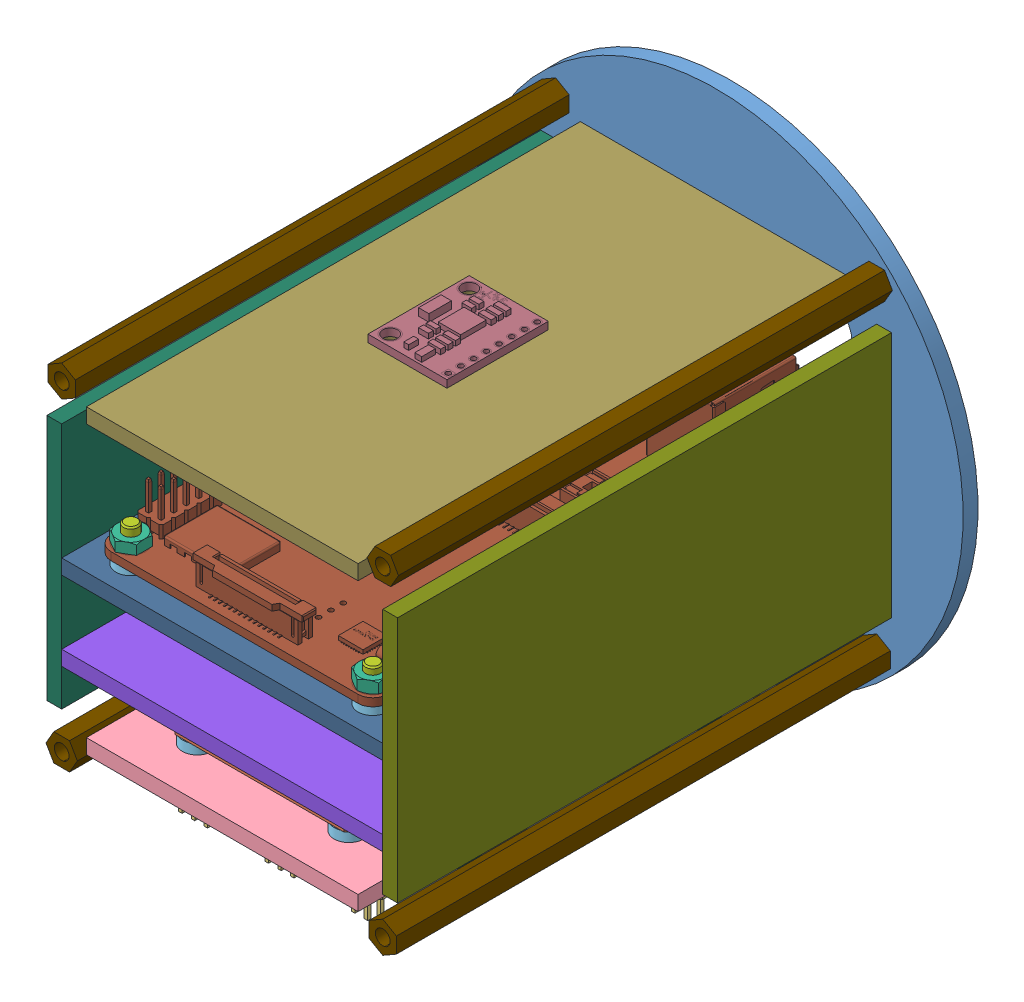
SolidWorks assembly Сборка4, configuration По умолчанию. Lengths in mm.
Overall size (100 100 104.65).
127 component instances, 20 part files, 170 mates.
Components (placement in the parent):
- baze-100mm-1: baze-100mm [По умолчанию] at origin size (100 100 3)
- Matek Power Hub-2: Matek Power Hub [По умолчанию] at (0.0123 -25.5 28.6623) x (0 0 -1) z (1 0 0) size (36.25 3.92 36.25)
- ACS712.step-1: ACS712.step [По умолчанию] at (17.5 -32.5 27.745) x (0 0 1) z (1 0 0) size (31.19 12.78 13.3)
- ACS712.step-2: ACS712.step [По умолчанию] at (0 -32.5 27.745) x (0 0 1) z (1 0 0) size (31.19 12.78 13.3)
- ACS712.step-3: ACS712.step [По умолчанию] at (-17.5 -32.5 27.745) x (0 0 1) z (1 0 0) size (31.19 12.78 13.3)
- level-0-1: level-0 [По умолчанию] at (0 -30.5 53) x (1 0 0) z (0 1 0) size (55 103 3)
- Matek Power Hub-4: Matek Power Hub [По умолчанию] at (0.0123 -25.5 77.3623) size (36.25 3.92 36.25)
- ACS712.step-7: ACS712.step [По умолчанию] at (17.5 -32.5 78.255) x (0 0 -1) z (-1 0 0) size (31.19 12.78 13.3)
- ACS712.step-8: ACS712.step [По умолчанию] at (0 -32.5 78.255) x (0 0 -1) z (-1 0 0) size (31.19 12.78 13.3)
- ACS712.step-9: ACS712.step [По умолчанию] at (-17.5 -32.5 78.255) x (0 0 -1) z (-1 0 0) size (31.19 12.78 13.3)
- 3-6-3-1: 3-6-3 [По умолчанию] at (15.35 -27.5 92.7) x (0.999975 0 -0.007062) z (0 1 0) size (6 6 2)
- 3-6-3-2: 3-6-3 [По умолчанию] at (-15.35 -27.5 92.7) x (0.992437 0 -0.122755) z (0 1 0) size (6 6 2)
- 3-6-3-3: 3-6-3 [По умолчанию] at (15.35 -27.5 62) x (0.931904 0 -0.362706) z (0 1 0) size (6 6 2)
- 3-6-3-4: 3-6-3 [По умолчанию] at (-15.35 -27.5 62) x (1 0 0) z (0 1 0) size (6 6 2)
- hex nut style 1 gradeab_iso-1: hex nut style 1 gradeab_iso [ISO - 4032 - M3 - D - N] at (15.3745 -21.9 62) x (1 0 0) z (0 1 0) size (5.5 6.35 2.4)
- hex nut style 1 gradeab_iso-2: hex nut style 1 gradeab_iso [ISO - 4032 - M3 - D - N] at (-15.35 -21.9 62) x (1 0 0) z (0 1 0) size (5.5 6.35 2.4)
- hex nut style 1 gradeab_iso-3: hex nut style 1 gradeab_iso [ISO - 4032 - M3 - D - N] at (15.3745 -21.9 92.7245) x (1 0 0) z (0 1 0) size (5.5 6.35 2.4)
- hex nut style 1 gradeab_iso-4: hex nut style 1 gradeab_iso [ISO - 4032 - M3 - D - N] at (-15.35 -21.9 92.7245) x (1 0 0) z (0 1 0) size (5.5 6.35 2.4)
- hex nut style 1 gradeab_iso-5: hex nut style 1 gradeab_iso [ISO - 4032 - M3 - D - N] at (15.3745 -21.9 44.0245) x (1 0 0) z (0 1 0) size (5.5 6.35 2.4)
- hex nut style 1 gradeab_iso-6: hex nut style 1 gradeab_iso [ISO - 4032 - M3 - D - N] at (-15.35 -21.9 44.0245) x (1 0 0) z (0 1 0) size (5.5 6.35 2.4)
- hex nut style 1 gradeab_iso-7: hex nut style 1 gradeab_iso [ISO - 4032 - M3 - D - N] at (15.3745 -21.9 13.3) x (1 0 0) z (0 1 0) size (5.5 6.35 2.4)
- hex nut style 1 gradeab_iso-8: hex nut style 1 gradeab_iso [ISO - 4032 - M3 - D - N] at (-15.35 -21.9 13.3) x (1 0 0) z (0 1 0) size (5.5 6.35 2.4)
- socket countersunk head screw_iso-1: socket countersunk head screw_iso [ISO 10642 - M3 x 8 - 8N] at (15.35 -30.11 92.7) x (0 1 0) z (-0.074206 0 0.997243) size (8 5.54 5.54)
- socket countersunk head screw_iso-2: socket countersunk head screw_iso [ISO 10642 - M3 x 8 - 8N] at (15.35 -30.11 62) x (0 1 0) z (-0.12314 0 0.992389) size (8 5.54 5.54)
- socket countersunk head screw_iso-3: socket countersunk head screw_iso [ISO 10642 - M3 x 8 - 8N] at (-15.35 -30.11 62) x (0 1 0) z (-0.109262 0 0.994013) size (8 5.54 5.54)
- socket countersunk head screw_iso-4: socket countersunk head screw_iso [ISO 10642 - M3 x 8 - 8N] at (-15.35 -30.11 92.7) x (0 1 0) z (-0.069269 0 0.997598) size (8 5.54 5.54)
- socket countersunk head screw_iso-5: socket countersunk head screw_iso [ISO 10642 - M3 x 8 - 8N] at (-22.5 -27.89 77.35) x (0 -1 0) z (-0.066693 0 0.997774) size (8 5.54 5.54)
- socket countersunk head screw_iso-6: socket countersunk head screw_iso [ISO 10642 - M3 x 8 - 8N] at (-12.5 -27.89 77.35) x (0 -1 0) z (-0.00561 0 0.999984) size (8 5.54 5.54)
- socket countersunk head screw_iso-7: socket countersunk head screw_iso [ISO 10642 - M3 x 8 - 8N] at (-5 -27.89 77.35) x (0 -1 0) z (0.004518 0 0.99999) size (8 5.54 5.54)
- socket countersunk head screw_iso-8: socket countersunk head screw_iso [ISO 10642 - M3 x 8 - 8N] at (5 -27.89 77.35) x (0 -1 0) z (0.047845 0 0.998855) size (8 5.54 5.54)
- socket countersunk head screw_iso-9: socket countersunk head screw_iso [ISO 10642 - M3 x 8 - 8N] at (12.5 -27.89 77.35) x (0 -1 0) z (0.031705 0 0.999497) size (8 5.54 5.54)
- socket countersunk head screw_iso-10: socket countersunk head screw_iso [ISO 10642 - M3 x 8 - 8N] at (22.5 -27.89 77.35) x (0 -1 0) z (0.037692 0 0.999289) size (8 5.54 5.54)
- hex nut style 1 gradeab_iso-13: hex nut style 1 gradeab_iso [ISO - 4032 - M3 - D - N] at (22.5 -36.48 77.35) x (1 0 0) z (0 -1 0) size (5.5 6.35 2.4)
- hex nut style 1 gradeab_iso-14: hex nut style 1 gradeab_iso [ISO - 4032 - M3 - D - N] at (12.5 -36.48 77.35) x (1 0 0) z (0 -1 0) size (5.5 6.35 2.4)
- hex nut style 1 gradeab_iso-15: hex nut style 1 gradeab_iso [ISO - 4032 - M3 - D - N] at (5 -36.48 77.35) x (1 0 0) z (0 -1 0) size (5.5 6.35 2.4)
- hex nut style 1 gradeab_iso-16: hex nut style 1 gradeab_iso [ISO - 4032 - M3 - D - N] at (-5 -36.48 77.35) x (1 0 0) z (0 -1 0) size (5.5 6.35 2.4)
- hex nut style 1 gradeab_iso-17: hex nut style 1 gradeab_iso [ISO - 4032 - M3 - D - N] at (-12.5 -36.48 77.35) x (1 0 0) z (0 -1 0) size (5.5 6.35 2.4)
- hex nut style 1 gradeab_iso-18: hex nut style 1 gradeab_iso [ISO - 4032 - M3 - D - N] at (-22.5 -36.48 77.35) x (1 0 0) z (0 -1 0) size (5.5 6.35 2.4)
- 3-6-3-5: 3-6-3 [По умолчанию] at (22.5 -32.5 77.35) x (1 0 0) z (0 1 0) size (6 6 2)
- 3-6-3-6: 3-6-3 [По умолчанию] at (12.5 -32.5 77.35) x (1 0 0) z (0 1 0) size (6 6 2)
- 3-6-3-7: 3-6-3 [По умолчанию] at (5 -32.5 77.35) x (1 0 0) z (0 1 0) size (6 6 2)
- 3-6-3-8: 3-6-3 [По умолчанию] at (-5 -32.5 77.35) x (1 0 0) z (0 1 0) size (6 6 2)
- 3-6-3-9: 3-6-3 [По умолчанию] at (-12.5 -32.5 77.35) x (1 0 0) z (0 1 0) size (6 6 2)
- 3-6-3-10: 3-6-3 [По умолчанию] at (-22.5 -32.5 77.35) x (1 0 0) z (0 1 0) size (6 6 2)
- 3-6-3-11: 3-6-3 [По умолчанию] at (-22.5 -30.5 28.65) x (1 0 0) z (0 -1 0) size (6 6 2)
- hex nut style 1 gradeab_iso-19: hex nut style 1 gradeab_iso [ISO - 4032 - M3 - D - N] at (-22.5 -34.08 28.65) x (1 0 0) z (0 1 0) size (5.5 6.35 2.4)
- hex nut style 1 gradeab_iso-20: hex nut style 1 gradeab_iso [ISO - 4032 - M3 - D - N] at (-12.5 -34.08 28.65) x (1 0 0) z (0 1 0) size (5.5 6.35 2.4)
- 3-6-3-12: 3-6-3 [По умолчанию] at (-12.5 -30.5 28.65) x (1 0 0) z (0 -1 0) size (6 6 2)
- hex nut style 1 gradeab_iso-21: hex nut style 1 gradeab_iso [ISO - 4032 - M3 - D - N] at (-5 -34.08 28.65) x (1 0 0) z (0 1 0) size (5.5 6.35 2.4)
- hex nut style 1 gradeab_iso-22: hex nut style 1 gradeab_iso [ISO - 4032 - M3 - D - N] at (5 -34.08 28.65) x (1 0 0) z (0 1 0) size (5.5 6.35 2.4)
- hex nut style 1 gradeab_iso-23: hex nut style 1 gradeab_iso [ISO - 4032 - M3 - D - N] at (12.5 -34.08 28.65) x (1 0 0) z (0 1 0) size (5.5 6.35 2.4)
- hex nut style 1 gradeab_iso-24: hex nut style 1 gradeab_iso [ISO - 4032 - M3 - D - N] at (22.5 -34.08 28.65) x (1 0 0) z (0 1 0) size (5.5 6.35 2.4)
- socket countersunk head screw_iso-11: socket countersunk head screw_iso [ISO 10642 - M3 x 8 - 8N] at (22.5 -27.89 28.65) x (0 -1 0) z (-0.037692 0 0.999289) size (8 5.54 5.54)
- socket countersunk head screw_iso-12: socket countersunk head screw_iso [ISO 10642 - M3 x 8 - 8N] at (12.5 -27.89 28.65) x (0 -1 0) z (-0.031705 0 0.999497) size (8 5.54 5.54)
- socket countersunk head screw_iso-13: socket countersunk head screw_iso [ISO 10642 - M3 x 8 - 8N] at (5 -27.89 28.65) x (0 -1 0) z (-0.047845 0 0.998855) size (8 5.54 5.54)
- socket countersunk head screw_iso-14: socket countersunk head screw_iso [ISO 10642 - M3 x 8 - 8N] at (-5 -27.89 28.65) x (0 -1 0) z (-0.004518 0 0.99999) size (8 5.54 5.54)
- socket countersunk head screw_iso-15: socket countersunk head screw_iso [ISO 10642 - M3 x 8 - 8N] at (-12.5 -27.89 28.65) x (0 -1 0) z (0.00561 0 0.999984) size (8 5.54 5.54)
- socket countersunk head screw_iso-16: socket countersunk head screw_iso [ISO 10642 - M3 x 8 - 8N] at (-22.5 -27.89 28.65) x (0 -1 0) z (0.066693 0 0.997774) size (8 5.54 5.54)
- 3-6-3-13: 3-6-3 [По умолчанию] at (-5 -30.5 28.65) x (1 0 0) z (0 -1 0) size (6 6 2)
- 3-6-3-14: 3-6-3 [По умолчанию] at (5 -30.5 28.65) x (1 0 0) z (0 -1 0) size (6 6 2)
- 3-6-3-15: 3-6-3 [По умолчанию] at (12.5 -30.5 28.65) x (1 0 0) z (0 -1 0) size (6 6 2)
- 3-6-3-16: 3-6-3 [По умолчанию] at (22.5 -30.5 28.65) x (1 0 0) z (0 -1 0) size (6 6 2)
- socket countersunk head screw_iso-17: socket countersunk head screw_iso [ISO 10642 - M3 x 8 - 8N] at (-15.35 -30.11 13.3) x (0 1 0) z (0.069269 0 0.997598) size (8 5.54 5.54)
- socket countersunk head screw_iso-18: socket countersunk head screw_iso [ISO 10642 - M3 x 8 - 8N] at (15.35 -30.11 13.3) x (0 1 0) z (0.074206 0 0.997243) size (8 5.54 5.54)
- socket countersunk head screw_iso-19: socket countersunk head screw_iso [ISO 10642 - M3 x 8 - 8N] at (-15.35 -30.11 44) x (0 1 0) z (0.109262 0 0.994013) size (8 5.54 5.54)
- socket countersunk head screw_iso-20: socket countersunk head screw_iso [ISO 10642 - M3 x 8 - 8N] at (15.35 -30.11 44) x (0 1 0) z (0.12314 0 0.992389) size (8 5.54 5.54)
- 3-6-3-17: 3-6-3 [По умолчанию] at (-15.35 -25.5 44) x (1 0 0) z (0 -1 0) size (6 6 2)
- 3-6-3-18: 3-6-3 [По умолчанию] at (-15.35 -25.5 13.3) x (0.992437 0 0.122755) z (0 -1 0) size (6 6 2)
- 3-6-3-19: 3-6-3 [По умолчанию] at (15.35 -25.5 44) x (0.931904 0 0.362706) z (0 -1 0) size (6 6 2)
- 3-6-3-20: 3-6-3 [По умолчанию] at (15.35 -25.5 13.3) x (0.999975 0 0.007062) z (0 -1 0) size (6 6 2)
- level-1-1: level-1 [По умолчанию] at (0 -17.5 53) x (1 0 0) z (0 1 0) size (65 103 3)
- 12Channel PWM-3: 12Channel PWM [Default] at (-16.4 -12.5 53) size (25.4 7.55 66.7)
- 12Channel PWM-4: 12Channel PWM [Default] at (16.4 -12.5 53) size (25.4 7.55 66.7)
- 3-6-3-21: 3-6-3 [По умолчанию] at (-25.8 -14.5 80.95) x (0.999704 0 0.024339) z (0 1 0) size (6 6 2)
- 3-6-3-22: 3-6-3 [По умолчанию] at (-7 -14.5 80.95) x (1 0 0) z (0 1 0) size (6 6 2)
- 3-6-3-23: 3-6-3 [По умолчанию] at (7 -14.5 80.95) x (1 0 0) z (0 1 0) size (6 6 2)
- 3-6-3-24: 3-6-3 [По умолчанию] at (25.8 -14.5 80.95) x (1 0 0) z (0 1 0) size (6 6 2)
- 3-6-3-25: 3-6-3 [По умолчанию] at (-25.8 -14.5 25.05) x (1 0 0) z (0 1 0) size (6 6 2)
- 3-6-3-26: 3-6-3 [По умолчанию] at (-7 -14.5 25.05) x (1 0 0) z (0 1 0) size (6 6 2)
- 3-6-3-27: 3-6-3 [По умолчанию] at (7 -14.5 25.05) x (1 0 0) z (0 1 0) size (6 6 2)
- 3-6-3-28: 3-6-3 [По умолчанию] at (25.8 -14.5 25.05) x (1 0 0) z (0 1 0) size (6 6 2)
- hex nut style 1 gradeab_iso-25: hex nut style 1 gradeab_iso [ISO - 4032 - M3 - D - N] at (25.8 -8.59 80.95) x (1 0 0) z (0 1 0) size (5.5 6.35 2.4)
- hex nut style 1 gradeab_iso-26: hex nut style 1 gradeab_iso [ISO - 4032 - M3 - D - N] at (7 -8.59 80.95) x (1 0 0) z (0 1 0) size (5.5 6.35 2.4)
- hex nut style 1 gradeab_iso-27: hex nut style 1 gradeab_iso [ISO - 4032 - M3 - D - N] at (-7 -8.59 80.95) x (1 0 0) z (0 1 0) size (5.5 6.35 2.4)
- hex nut style 1 gradeab_iso-28: hex nut style 1 gradeab_iso [ISO - 4032 - M3 - D - N] at (-25.8 -8.59 80.95) x (1 0 0) z (0 1 0) size (5.5 6.35 2.4)
- hex nut style 1 gradeab_iso-29: hex nut style 1 gradeab_iso [ISO - 4032 - M3 - D - N] at (-7 -8.6 25.05) x (1 0 0) z (0 1 0) size (5.5 6.35 2.4)
- hex nut style 1 gradeab_iso-30: hex nut style 1 gradeab_iso [ISO - 4032 - M3 - D - N] at (-25.8 -8.59 25.05) x (1 0 0) z (0 1 0) size (5.5 6.35 2.4)
- hex nut style 1 gradeab_iso-31: hex nut style 1 gradeab_iso [ISO - 4032 - M3 - D - N] at (25.8 -8.59 25.05) x (1 0 0) z (0 1 0) size (5.5 6.35 2.4)
- hex nut style 1 gradeab_iso-32: hex nut style 1 gradeab_iso [ISO - 4032 - M3 - D - N] at (7 -8.59 25.05) x (1 0 0) z (0 1 0) size (5.5 6.35 2.4)
- socket countersunk head screw_iso-21: socket countersunk head screw_iso [ISO 10642 - M3 x 10 - 10N] at (25.8 -17.11 80.95) x (0 1 0) z (-0.063472 0 0.997984) size (10 5.54 5.54)
- socket countersunk head screw_iso-22: socket countersunk head screw_iso [ISO 10642 - M3 x 10 - 10N] at (7 -17.11 80.95) x (0 1 0) z (-0.051642 0 0.998666) size (10 5.54 5.54)
- socket countersunk head screw_iso-23: socket countersunk head screw_iso [ISO 10642 - M3 x 10 - 10N] at (25.8 -17.11 25.05) x (0 1 0) z (-0.110304 0 0.993898) size (10 5.54 5.54)
- socket countersunk head screw_iso-24: socket countersunk head screw_iso [ISO 10642 - M3 x 10 - 10N] at (7 -17.11 25.05) x (0 1 0) z (-0.201092 0 0.979572) size (10 5.54 5.54)
- socket countersunk head screw_iso-25: socket countersunk head screw_iso [ISO 10642 - M3 x 10 - 10N] at (-25.8 -17.11 25.05) x (0 1 0) z (0.159633 0 0.987176) size (10 5.54 5.54)
- socket countersunk head screw_iso-26: socket countersunk head screw_iso [ISO 10642 - M3 x 10 - 10N] at (-25.8 -17.11 80.95) x (0 1 0) z (-0.028986 0 0.99958) size (10 5.54 5.54)
- socket countersunk head screw_iso-27: socket countersunk head screw_iso [ISO 10642 - M3 x 10 - 10N] at (-7 -17.11 80.95) x (0 1 0) z (0.071549 0 0.997437) size (10 5.54 5.54)
- socket countersunk head screw_iso-28: socket countersunk head screw_iso [ISO 10642 - M3 x 10 - 10N] at (-7 -17.11 25.05) x (0 1 0) z (0.217599 0 0.976038) size (10 5.54 5.54)
- level-2-1: level-2 [По умолчанию] at (0 -1.5 53) x (1 0 0) z (0 1 0) size (65 103 3)
- Raspberry Pi 4 Model B-2: Raspberry Pi 4 Model B [По умолчанию] at (0 4.3 58) x (0 0 -1) z (1 0 0) size (88.99 19.91 58.4)
- 3-6-3-29: 3-6-3 [По умолчанию] at (24.5 1.5 97) x (0.990055 0 0.140681) z (0 1 0) size (6 6 2)
- 3-6-3-30: 3-6-3 [По умолчанию] at (-24.5 1.5 97) x (1 0 0) z (0 1 0) size (6 6 2)
- 3-6-3-31: 3-6-3 [По умолчанию] at (24.5 1.5 39) x (1 0 0) z (0 1 0) size (6 6 2)
- 3-6-3-32: 3-6-3 [По умолчанию] at (-24.5 1.5 39) x (1 0 0) z (0 1 0) size (6 6 2)
- socket countersunk head screw_iso-29: socket countersunk head screw_iso [ISO 10642 - M3 x 10 - 10N] at (24.5 -1.11 97) x (0 1 0) z (0.024362 0 0.999703) size (10 5.54 5.54)
- socket countersunk head screw_iso-30: socket countersunk head screw_iso [ISO 10642 - M3 x 10 - 10N] at (-24.5 -1.11 97) x (0 1 0) z (0.004569 0 0.99999) size (10 5.54 5.54)
- socket countersunk head screw_iso-31: socket countersunk head screw_iso [ISO 10642 - M3 x 10 - 10N] at (-24.5 -1.11 39) x (0 1 0) z (0.093979 0 0.995574) size (10 5.54 5.54)
- socket countersunk head screw_iso-32: socket countersunk head screw_iso [ISO 10642 - M3 x 10 - 10N] at (24.5 -1.11 39) x (0 1 0) z (-0.034666 0 0.999399) size (10 5.54 5.54)
- hex nut style 1 gradeab_iso-33: hex nut style 1 gradeab_iso [ISO - 4032 - M3 - D - N] at (-24.5 4.787 97) x (1 0 0) z (0 -1 0) size (5.5 6.35 2.4)
- hex nut style 1 gradeab_iso-34: hex nut style 1 gradeab_iso [ISO - 4032 - M3 - D - N] at (-24.5 7.49 39) x (1 0 0) z (0 1 0) size (5.5 6.35 2.4)
- hex nut style 1 gradeab_iso-35: hex nut style 1 gradeab_iso [ISO - 4032 - M3 - D - N] at (24.5 7.49 97) x (1 0 0) z (0 1 0) size (5.5 6.35 2.4)
- hex nut style 1 gradeab_iso-36: hex nut style 1 gradeab_iso [ISO - 4032 - M3 - D - N] at (24.5 7.49 39) x (1 0 0) z (0 1 0) size (5.5 6.35 2.4)
- level-3-1: level-3 [По умолчанию] at (0 27.5 53) x (1 0 0) z (0 1 0) size (55 103 3)
- MPU_6050-1: MPU_6050 [По умолчанию] at (-2.25 32 53) x (0 0 -1) z (0 1 0) size (20.5 16 3)
- radiator-1: radiator [Standard] at (-3.916 7.5 71.0007) size (12 12.1 15)
- level-4-1: level-4 [По умолчанию] at (-32.4957 0 53) x (0 1 0) z (-1 0 0) size (50 103 3)
- level-5-1: level-5 [По умолчанию] at (32.4957 0 53) x (0 -1 0) z (1 0 0) size (50 103 3)
- 16Bit I2C ADC+PGA - ADS1115-1: 16Bit I2C ADC+PGA - ADS1115 [По умолчанию] at (-37.5034 -13.6367 30.8709) x (0 0 1) z (-1 0 0) size (27.94 17.27 2.74)
- 16Bit I2C ADC+PGA - ADS1115-2: 16Bit I2C ADC+PGA - ADS1115 [По умолчанию] at (-36.9561 -12.9358 66.9922) x (0 0 1) z (-1 0 0) size (27.94 17.27 2.74)
- 3-100-1: 3-100 [По умолчанию] at (32.5 32.5 3) size (6.35 5.5 100)
- 3-100-2: 3-100 [По умолчанию] at (32.5 -32.5 3) x (0 -1 0) z (0 0 1) size (6.35 5.5 100)
- 3-100-3: 3-100 [По умолчанию] at (-32.5 -32.5 3) x (-1 0 0) z (0 0 1) size (6.35 5.5 100)
- 3-100-4: 3-100 [По умолчанию] at (-32.5 32.5 3) x (0 1 0) z (0 0 1) size (6.35 5.5 100)
- socket button head screw_iso-3: socket button head screw_iso [ISO 7380 - M3 x 10 - 10N] at (32.5 -32.5 -1.65) x (0 0 1) z (-1 0 0) size (11.65 5.7 5.7)
- socket button head screw_iso-4: socket button head screw_iso [ISO 7380 - M3 x 10 - 10N] at (-32.5 -32.5 -1.65) x (0 0 1) z (-1 0 0) size (11.65 5.7 5.7)
- socket button head screw_iso-5: socket button head screw_iso [ISO 7380 - M3 x 10 - 10N] at (32.5 32.5 -1.65) x (0 0 1) z (-1 0 0) size (11.65 5.7 5.7)
- socket button head screw_iso-6: socket button head screw_iso [ISO 7380 - M3 x 10 - 10N] at (-32.5 32.5 -1.65) x (0 0 1) z (-1 0 0) size (11.65 5.7 5.7)
- 20-80-shild-1: 20-80-shild [По умолчанию] at (-37.308 7.7953 49.1272) x (0 0 -1) z (1 0 0) size (80 20 1.6)
Mates (geometry in assembly coordinates):
- Совпадение1: coincident anti-aligned: plane of baze-100mm-1 through (-15 -27.5 -5) normal (0 -1 0); plane of level-0-1 through (0 -27.5 53) normal (0 1 0)
- Совпадение2: coincident anti-aligned: plane of baze-100mm-1 through (0 0 3) normal (0 0 1); plane of level-0-1 through (0 -27.5 3) normal (0 0 -1)
- Совпадение3: coincident anti-aligned: plane of baze-100mm-1 through (15 -27.5 -5) normal (-1 0 0); plane of level-0-1 through (15 -27.5 53) normal (1 0 0)
- Концентричный1: concentric anti-aligned: cylinder of Matek Power Hub-2 through (-15.35 -24.3 13.3) axis (0 -1 0) radius 1.75; cylinder of level-0-1 through (-15.35 -37.5 13.3) axis (0 1 0) radius 1.75
- Параллельность1: parallel aligned: plane of Matek Power Hub-2 through (-18.1127 -25.5 10.5373) normal (-1 0 0); plane of level-0-1 through (-27.5 -27.5 53) normal (-1 0 0)
- Концентричный2: concentric anti-aligned: cylinder of level-0-1 through (-15.35 -37.5 62) axis (0 1 0) radius 1.75; cylinder of Matek Power Hub-4 through (-15.35 -24.3 62) axis (0 -1 0) radius 1.75
- Параллельность2: parallel aligned: plane of level-0-1 through (-27.5 -27.5 53) normal (-1 0 0); plane of Matek Power Hub-4 through (-18.1127 -25.5 59.2373) normal (-1 0 0)
- Совпадение7: coincident aligned: plane of Matek Power Hub-2 through (0.0123 -24.3 28.6623) normal (0 1 0); plane of Matek Power Hub-4 through (0.0123 -24.3 77.3623) normal (0 1 0)
- Параллельность4: parallel aligned: plane of ACS712.step-1 through (24.15 -34.08 12.15) normal (1 0 0); plane of level-0-1 through (27.5 -27.5 53) normal (1 0 0)
- Параллельность5: parallel anti-aligned: plane of ACS712.step-1 through (17.5 -32.5 27.745) normal (0 1 0); plane of level-0-1 through (0 -30.5 53) normal (0 -1 0)
- Концентричный5: concentric anti-aligned: cylinder of ACS712.step-3 through (-22.5 -44.08 28.65) axis (0 1 0) radius 1.5; cylinder of level-0-1 through (-22.5 -20.5 28.65) axis (0 -1 0) radius 1.75
- Концентричный6: concentric anti-aligned: cylinder of level-0-1 through (22.5 -20.5 77.35) axis (0 -1 0) radius 1.75; cylinder of ACS712.step-7 through (22.5 -44.08 77.35) axis (0 1 0) radius 1.5
- Параллельность6: parallel aligned: plane of level-0-1 through (27.5 -27.5 53) normal (1 0 0); plane of ACS712.step-7 through (24.15 -34.08 93.85) normal (1 0 0)
- Совпадение13: coincident aligned: plane of ACS712.step-3 through (-17.5 -34.08 27.745) normal (0 -1 0); plane of ACS712.step-9 through (-17.5 -34.08 78.255) normal (0 -1 0)
- Концентричный7: concentric anti-aligned: cylinder of level-0-1 through (15.35 -37.5 92.7) axis (0 1 0) radius 1.75; cylinder of 3-6-3-1 through (15.35 -25.5 92.7) axis (0 -1 0) radius 1.75
- Совпадение14: coincident anti-aligned: plane of level-0-1 through (0 -27.5 53) normal (0 1 0); plane of 3-6-3-1 through (15.35 -27.5 92.7) normal (0 -1 0)
- Концентричный8: concentric anti-aligned: cylinder of level-0-1 through (-15.35 -37.5 92.7) axis (0 1 0) radius 1.75; cylinder of 3-6-3-2 through (-15.35 -25.5 92.7) axis (0 -1 0) radius 1.75
- Совпадение15: coincident anti-aligned: plane of level-0-1 through (0 -27.5 53) normal (0 1 0); plane of 3-6-3-2 through (-15.35 -27.5 92.7) normal (0 -1 0)
- Концентричный9: concentric anti-aligned: cylinder of level-0-1 through (15.35 -37.5 62) axis (0 1 0) radius 1.75; cylinder of 3-6-3-3 through (15.35 -25.5 62) axis (0 -1 0) radius 1.75
- Совпадение16: coincident anti-aligned: plane of level-0-1 through (0 -27.5 53) normal (0 1 0); plane of 3-6-3-3 through (15.35 -27.5 62) normal (0 -1 0)
- Концентричный10: concentric anti-aligned: cylinder of level-0-1 through (-15.35 -37.5 62) axis (0 1 0) radius 1.75; cylinder of 3-6-3-4 through (-15.35 -25.5 62) axis (0 -1 0) radius 1.75
- Совпадение17: coincident anti-aligned: plane of Matek Power Hub-4 through (0.0123 -25.5 77.3623) normal (0 -1 0); plane of 3-6-3-4 through (-15.35 -25.5 62) normal (0 1 0)
- Совпадение18: coincident anti-aligned: plane of level-0-1 through (0 -27.5 53) normal (0 1 0); plane of 3-6-3-4 through (-15.35 -27.5 62) normal (0 -1 0)
- Концентричный12: concentric anti-aligned: cylinder of Matek Power Hub-4 through (15.3745 -24.3 62) axis (0 -1 0) radius 1.75; cylinder of hex nut style 1 gradeab_iso-1 through (15.3745 -46.9375 62) axis (0 1 0) radius 1.5
- Совпадение20: coincident anti-aligned: plane of Matek Power Hub-4 through (15.3745 -24.3 62) normal (0 1 0); plane of hex nut style 1 gradeab_iso-1 through (15.3745 -24.3 58.8246) normal (0 -1 0)
- Концентричный13: concentric anti-aligned: cylinder of Matek Power Hub-4 through (-15.35 -24.3 62) axis (0 -1 0) radius 1.75; cylinder of hex nut style 1 gradeab_iso-2 through (-15.35 -46.9375 62) axis (0 1 0) radius 1.5
- Совпадение21: coincident anti-aligned: plane of Matek Power Hub-4 through (-15.35 -24.3 62) normal (0 1 0); plane of hex nut style 1 gradeab_iso-2 through (-15.35 -24.3 58.8246) normal (0 -1 0)
- Концентричный14: concentric anti-aligned: cylinder of Matek Power Hub-4 through (15.3745 -24.3 92.7245) axis (0 -1 0) radius 2; cylinder of hex nut style 1 gradeab_iso-3 through (15.3745 -46.9375 92.7245) axis (0 1 0) radius 1.5
- Совпадение22: coincident anti-aligned: plane of Matek Power Hub-4 through (0.0123 -24.3 77.3623) normal (0 1 0); plane of hex nut style 1 gradeab_iso-3 through (15.3745 -24.3 89.5491) normal (0 -1 0)
- Концентричный15: concentric anti-aligned: cylinder of Matek Power Hub-4 through (-15.35 -24.3 92.7245) axis (0 -1 0) radius 2; cylinder of hex nut style 1 gradeab_iso-4 through (-15.35 -46.9375 92.7245) axis (0 1 0) radius 1.5
- Совпадение23: coincident anti-aligned: plane of Matek Power Hub-4 through (0.0123 -24.3 77.3623) normal (0 1 0); plane of hex nut style 1 gradeab_iso-4 through (-15.35 -24.3 89.5491) normal (0 -1 0)
- Концентричный16: concentric anti-aligned: cylinder of Matek Power Hub-2 through (15.3745 -24.3 44.0245) axis (0 -1 0) radius 1.75; cylinder of hex nut style 1 gradeab_iso-5 through (15.3745 -46.9375 44.0245) axis (0 1 0) radius 1.5
- Совпадение24: coincident anti-aligned: plane of Matek Power Hub-2 through (15.3745 -24.3 44.0245) normal (0 1 0); plane of hex nut style 1 gradeab_iso-5 through (15.3745 -24.3 40.8491) normal (0 -1 0)
- Концентричный17: concentric anti-aligned: cylinder of Matek Power Hub-2 through (-15.35 -24.3 44.0245) axis (0 -1 0) radius 2; cylinder of hex nut style 1 gradeab_iso-6 through (-15.35 -46.9375 44.0245) axis (0 1 0) radius 1.5
- Совпадение25: coincident anti-aligned: plane of Matek Power Hub-2 through (0.0123 -24.3 28.6623) normal (0 1 0); plane of hex nut style 1 gradeab_iso-6 through (-15.35 -24.3 40.8491) normal (0 -1 0)
- Концентричный18: concentric anti-aligned: cylinder of Matek Power Hub-2 through (15.3745 -24.3 13.3) axis (0 -1 0) radius 2; cylinder of hex nut style 1 gradeab_iso-7 through (15.3745 -46.9375 13.3) axis (0 1 0) radius 1.5
- Совпадение26: coincident anti-aligned: plane of Matek Power Hub-2 through (15.3745 -24.3 13.3) normal (0 1 0); plane of hex nut style 1 gradeab_iso-7 through (15.3745 -24.3 10.1246) normal (0 -1 0)
- Концентричный19: concentric anti-aligned: cylinder of Matek Power Hub-2 through (-15.35 -24.3 13.3) axis (0 -1 0) radius 1.75; cylinder of hex nut style 1 gradeab_iso-8 through (-15.35 -46.9375 13.3) axis (0 1 0) radius 1.5
- Совпадение27: coincident anti-aligned: plane of Matek Power Hub-2 through (-15.35 -24.3 13.3) normal (0 1 0); plane of hex nut style 1 gradeab_iso-8 through (-15.35 -24.3 10.1246) normal (0 -1 0)
- Совпадение28: coincident aligned: cone of level-0-1 through (15.35 -30.5 92.7) axis (0 1 0); cone of socket countersunk head screw_iso-1 through (15.35 -29.52 92.7) axis (0 1 0)
- Совпадение29: coincident aligned: cone of level-0-1 through (15.35 -30.5 62) axis (0 1 0); cone of socket countersunk head screw_iso-2 through (15.35 -29.52 62) axis (0 1 0)
- Совпадение30: coincident aligned: cone of level-0-1 through (-15.35 -30.5 62) axis (0 1 0); cone of socket countersunk head screw_iso-3 through (-15.35 -29.52 62) axis (0 1 0)
- Совпадение31: coincident aligned: cone of level-0-1 through (-15.35 -30.5 92.7) axis (0 1 0); cone of socket countersunk head screw_iso-4 through (-15.35 -29.52 92.7) axis (0 1 0)
- Совпадение32: coincident aligned: cone of level-0-1 through (-22.5 -29.5 77.35) axis (0 -1 0); cone of socket countersunk head screw_iso-5 through (-22.5 -28.48 77.35) axis (0 -1 0)
- Совпадение33: coincident aligned: cone of level-0-1 through (-12.5 -29.5 77.35) axis (0 -1 0); cone of socket countersunk head screw_iso-6 through (-12.5 -28.48 77.35) axis (0 -1 0)
- Совпадение34: coincident aligned: cone of level-0-1 through (-5 -29.5 77.35) axis (0 -1 0); cone of socket countersunk head screw_iso-7 through (-5 -28.48 77.35) axis (0 -1 0)
- Совпадение35: coincident aligned: cone of level-0-1 through (5 -29.5 77.35) axis (0 -1 0); cone of socket countersunk head screw_iso-8 through (5 -28.48 77.35) axis (0 -1 0)
- Совпадение36: coincident aligned: cone of level-0-1 through (12.5 -29.5 77.35) axis (0 -1 0); cone of socket countersunk head screw_iso-9 through (12.5 -28.48 77.35) axis (0 -1 0)
- Совпадение37: coincident aligned: cone of level-0-1 through (22.5 -29.5 77.35) axis (0 -1 0); cone of socket countersunk head screw_iso-10 through (22.5 -28.48 77.35) axis (0 -1 0)
- Концентричный23: concentric anti-aligned: cylinder of ACS712.step-7 through (22.5 -44.08 77.35) axis (0 1 0) radius 1.5; cylinder of hex nut style 1 gradeab_iso-13 through (22.5 -11.4425 77.35) axis (0 -1 0) radius 1.5
- Совпадение41: coincident anti-aligned: plane of ACS712.step-7 through (17.5 -34.08 78.255) normal (0 -1 0); plane of hex nut style 1 gradeab_iso-13 through (22.5 -34.08 80.5254) normal (0 1 0)
- Концентричный24: concentric anti-aligned: cylinder of ACS712.step-7 through (12.5 -44.08 77.35) axis (0 1 0) radius 1.5; cylinder of hex nut style 1 gradeab_iso-14 through (12.5 -11.4425 77.35) axis (0 -1 0) radius 1.5
- Совпадение42: coincident anti-aligned: plane of ACS712.step-7 through (17.5 -34.08 78.255) normal (0 -1 0); plane of hex nut style 1 gradeab_iso-14 through (12.5 -34.08 80.5254) normal (0 1 0)
- Концентричный25: concentric anti-aligned: cylinder of ACS712.step-8 through (5 -44.08 77.35) axis (0 1 0) radius 1.5; cylinder of hex nut style 1 gradeab_iso-15 through (5 -11.4425 77.35) axis (0 -1 0) radius 1.5
- Совпадение43: coincident anti-aligned: plane of ACS712.step-8 through (0 -34.08 78.255) normal (0 -1 0); plane of hex nut style 1 gradeab_iso-15 through (5 -34.08 80.5254) normal (0 1 0)
- Концентричный26: concentric anti-aligned: cylinder of ACS712.step-8 through (-5 -44.08 77.35) axis (0 1 0) radius 1.5; cylinder of hex nut style 1 gradeab_iso-16 through (-5 -11.4425 77.35) axis (0 -1 0) radius 1.5
- Совпадение44: coincident anti-aligned: plane of ACS712.step-8 through (0 -34.08 78.255) normal (0 -1 0); plane of hex nut style 1 gradeab_iso-16 through (-5 -34.08 80.5254) normal (0 1 0)
- Концентричный27: concentric anti-aligned: cylinder of ACS712.step-9 through (-12.5 -44.08 77.35) axis (0 1 0) radius 1.5; cylinder of hex nut style 1 gradeab_iso-17 through (-12.5 -11.4425 77.35) axis (0 -1 0) radius 1.5
- Совпадение45: coincident anti-aligned: plane of ACS712.step-9 through (-17.5 -34.08 78.255) normal (0 -1 0); plane of hex nut style 1 gradeab_iso-17 through (-12.5 -34.08 80.5254) normal (0 1 0)
- Концентричный28: concentric anti-aligned: cylinder of ACS712.step-9 through (-22.5 -44.08 77.35) axis (0 1 0) radius 1.5; cylinder of hex nut style 1 gradeab_iso-18 through (-22.5 -11.4425 77.35) axis (0 -1 0) radius 1.5
- Совпадение46: coincident anti-aligned: plane of ACS712.step-9 through (-17.5 -34.08 78.255) normal (0 -1 0); plane of hex nut style 1 gradeab_iso-18 through (-22.5 -34.08 80.5254) normal (0 1 0)
- Концентричный29: concentric anti-aligned: cylinder of socket countersunk head screw_iso-10 through (22.5 -27.89 77.35) axis (0 1 0) radius 1.5; cylinder of 3-6-3-5 through (22.5 -30.5 77.35) axis (0 -1 0) radius 1.75
- Концентричный30: concentric anti-aligned: cylinder of socket countersunk head screw_iso-9 through (12.5 -27.89 77.35) axis (0 1 0) radius 1.5; cylinder of 3-6-3-6 through (12.5 -30.5 77.35) axis (0 -1 0) radius 1.75
- Концентричный31: concentric anti-aligned: cylinder of socket countersunk head screw_iso-8 through (5 -27.89 77.35) axis (0 1 0) radius 1.5; cylinder of 3-6-3-7 through (5 -30.5 77.35) axis (0 -1 0) radius 1.75
- Концентричный32: concentric anti-aligned: cylinder of socket countersunk head screw_iso-7 through (-5 -27.89 77.35) axis (0 1 0) radius 1.5; cylinder of 3-6-3-8 through (-5 -30.5 77.35) axis (0 -1 0) radius 1.75
- Концентричный33: concentric anti-aligned: cylinder of socket countersunk head screw_iso-6 through (-12.5 -27.89 77.35) axis (0 1 0) radius 1.5; cylinder of 3-6-3-9 through (-12.5 -30.5 77.35) axis (0 -1 0) radius 1.75
- Концентричный34: concentric anti-aligned: cylinder of socket countersunk head screw_iso-5 through (-22.5 -27.89 77.35) axis (0 1 0) radius 1.5; cylinder of 3-6-3-10 through (-22.5 -30.5 77.35) axis (0 -1 0) radius 1.75
- Совпадение47: coincident anti-aligned: plane of level-0-1 through (0 -30.5 53) normal (0 -1 0); plane of 3-6-3-5 through (22.5 -30.5 77.35) normal (0 1 0)
- Совпадение48: coincident anti-aligned: plane of level-0-1 through (0 -30.5 53) normal (0 -1 0); plane of 3-6-3-6 through (12.5 -30.5 77.35) normal (0 1 0)
- Совпадение49: coincident anti-aligned: plane of level-0-1 through (0 -30.5 53) normal (0 -1 0); plane of 3-6-3-7 through (5 -30.5 77.35) normal (0 1 0)
- Совпадение50: coincident anti-aligned: plane of level-0-1 through (0 -30.5 53) normal (0 -1 0); plane of 3-6-3-8 through (-5 -30.5 77.35) normal (0 1 0)
- Совпадение51: coincident anti-aligned: plane of level-0-1 through (0 -30.5 53) normal (0 -1 0); plane of 3-6-3-9 through (-12.5 -30.5 77.35) normal (0 1 0)
- Совпадение52: coincident anti-aligned: plane of level-0-1 through (0 -30.5 53) normal (0 -1 0); plane of 3-6-3-10 through (-22.5 -30.5 77.35) normal (0 1 0)
- Совпадение54: coincident anti-aligned: plane of ACS712.step-9 through (-17.5 -32.5 78.255) normal (0 1 0); plane of 3-6-3-10 through (-22.5 -32.5 77.35) normal (0 -1 0)
- Совпадение55: coincident anti-aligned: plane of baze-100mm-1 through (-17.5 -14.5 -5) normal (0 -1 0); plane of level-1-1 through (0 -14.5 53) normal (0 1 0)
- Совпадение56: coincident anti-aligned: plane of baze-100mm-1 through (0 0 3) normal (0 0 1); plane of level-1-1 through (0 -14.5 3) normal (0 0 -1)
- Совпадение57: coincident anti-aligned: plane of baze-100mm-1 through (-17.5 -14.5 -5) normal (1 0 0); plane of level-1-1 through (-17.5 -14.5 53) normal (-1 0 0)
- Концентричный35: concentric anti-aligned: cylinder of level-1-1 through (-25.8 -24.5 80.95) axis (0 1 0) radius 1.75; cylinder of 3-6-3-21 through (-25.8 -12.5 80.95) axis (0 -1 0) radius 1.75
- Концентричный36: concentric anti-aligned: cylinder of level-1-1 through (-7 -24.5 80.95) axis (0 1 0) radius 1.75; cylinder of 3-6-3-22 through (-7 -12.5 80.95) axis (0 -1 0) radius 1.75
- Концентричный37: concentric anti-aligned: cylinder of level-1-1 through (7 -24.5 80.95) axis (0 1 0) radius 1.75; cylinder of 3-6-3-23 through (7 -12.5 80.95) axis (0 -1 0) radius 1.75
- Концентричный38: concentric anti-aligned: cylinder of level-1-1 through (25.8 -24.5 80.95) axis (0 1 0) radius 1.75; cylinder of 3-6-3-24 through (25.8 -12.5 80.95) axis (0 -1 0) radius 1.75
- Концентричный39: concentric anti-aligned: cylinder of level-1-1 through (-25.8 -24.5 25.05) axis (0 1 0) radius 1.75; cylinder of 3-6-3-25 through (-25.8 -12.5 25.05) axis (0 -1 0) radius 1.75
- Концентричный40: concentric anti-aligned: cylinder of level-1-1 through (-7 -24.5 25.05) axis (0 1 0) radius 1.75; cylinder of 3-6-3-26 through (-7 -12.5 25.05) axis (0 -1 0) radius 1.75
- Концентричный41: concentric anti-aligned: cylinder of level-1-1 through (7 -24.5 25.05) axis (0 1 0) radius 1.75; cylinder of 3-6-3-27 through (7 -12.5 25.05) axis (0 -1 0) radius 1.75
- Концентричный42: concentric anti-aligned: cylinder of level-1-1 through (25.8 -24.5 25.05) axis (0 1 0) radius 1.75; cylinder of 3-6-3-28 through (25.8 -12.5 25.05) axis (0 -1 0) radius 1.75
- Совпадение58: coincident aligned: plane of 3-6-3-27 through (7 -12.5 25.05) normal (0 1 0); plane of 3-6-3-28 through (25.8 -12.5 25.05) normal (0 1 0)
- Совпадение59: coincident aligned: plane of 3-6-3-26 through (-7 -12.5 25.05) normal (0 1 0); plane of 3-6-3-27 through (7 -12.5 25.05) normal (0 1 0)
- Совпадение60: coincident aligned: plane of 3-6-3-25 through (-25.8 -12.5 25.05) normal (0 1 0); plane of 3-6-3-26 through (-7 -12.5 25.05) normal (0 1 0)
- Совпадение61: coincident aligned: plane of 3-6-3-21 through (-25.8 -12.5 80.95) normal (0 1 0); plane of 3-6-3-22 through (-7 -12.5 80.95) normal (0 1 0)
- Совпадение62: coincident aligned: plane of 3-6-3-22 through (-7 -12.5 80.95) normal (0 1 0); plane of 3-6-3-23 through (7 -12.5 80.95) normal (0 1 0)
- Совпадение63: coincident aligned: plane of 3-6-3-23 through (7 -12.5 80.95) normal (0 1 0); plane of 3-6-3-24 through (25.8 -12.5 80.95) normal (0 1 0)
- Совпадение64: coincident aligned: plane of 3-6-3-21 through (-25.8 -12.5 80.95) normal (0 1 0); plane of 3-6-3-25 through (-25.8 -12.5 25.05) normal (0 1 0)
- Совпадение65: coincident anti-aligned: plane of level-1-1 through (0 -14.5 53) normal (0 1 0); plane of 3-6-3-21 through (-25.8 -14.5 80.95) normal (0 -1 0)
- Концентричный43: concentric aligned: cylinder of level-1-1 through (-25.8 -24.5 80.95) axis (0 1 0) radius 1.75; cylinder of 12Channel PWM-3 through (-25.8 -16.0355 80.95) axis (0 1 0) radius 1.25
- Параллельность8: parallel aligned: plane of level-1-1 through (-32.5 -14.5 53) normal (-1 0 0); plane of 12Channel PWM-3 through (-29.1 -11 25.05) normal (-1 0 0)
- Концентричный44: concentric aligned: cylinder of level-1-1 through (25.8 -24.5 80.95) axis (0 1 0) radius 1.75; cylinder of 12Channel PWM-4 through (25.8 -16.0355 80.95) axis (0 1 0) radius 1.25
- Параллельность9: parallel aligned: plane of level-1-1 through (32.5 -14.5 53) normal (1 0 0); plane of 12Channel PWM-4 through (29.1 -11 25.05) normal (1 0 0)
- Совпадение68: coincident aligned: plane of 12Channel PWM-3 through (-7 -11 25.05) normal (0 1 0); plane of 12Channel PWM-4 through (25.8 -11 25.05) normal (0 1 0)
- Совпадение69: coincident anti-aligned: plane of 12Channel PWM-4 through (25.8 -12.5 25.05) normal (0 -1 0); plane of 3-6-3-24 through (25.8 -12.5 80.95) normal (0 1 0)
- Концентричный45: concentric aligned: cylinder of 12Channel PWM-4 through (25.8 -16.0355 80.95) axis (0 1 0) radius 1.25; cylinder of hex nut style 1 gradeab_iso-25 through (25.8 -33.6275 80.95) axis (0 1 0) radius 1.5
- Совпадение70: coincident anti-aligned: plane of 12Channel PWM-4 through (25.8 -10.99 80.95) normal (0 1 0); plane of hex nut style 1 gradeab_iso-25 through (25.8 -10.99 77.7746) normal (0 -1 0)
- Концентричный46: concentric aligned: cylinder of 12Channel PWM-4 through (7 -16.0355 80.95) axis (0 1 0) radius 1.25; cylinder of hex nut style 1 gradeab_iso-26 through (7 -33.6275 80.95) axis (0 1 0) radius 1.5
- Совпадение71: coincident anti-aligned: plane of 12Channel PWM-4 through (7 -10.99 80.95) normal (0 1 0); plane of hex nut style 1 gradeab_iso-26 through (7 -10.99 77.7746) normal (0 -1 0)
- Концентричный47: concentric aligned: cylinder of 12Channel PWM-3 through (-7 -16.0355 80.95) axis (0 1 0) radius 1.25; cylinder of hex nut style 1 gradeab_iso-27 through (-7 -33.6275 80.95) axis (0 1 0) radius 1.5
- Совпадение72: coincident anti-aligned: plane of 12Channel PWM-3 through (-7 -10.99 80.95) normal (0 1 0); plane of hex nut style 1 gradeab_iso-27 through (-7 -10.99 77.7746) normal (0 -1 0)
- Концентричный48: concentric aligned: cylinder of 12Channel PWM-3 through (-25.8 -16.0355 80.95) axis (0 1 0) radius 1.25; cylinder of hex nut style 1 gradeab_iso-28 through (-25.8 -33.6275 80.95) axis (0 1 0) radius 1.5
- Совпадение73: coincident anti-aligned: plane of 12Channel PWM-3 through (-25.8 -10.99 80.95) normal (0 1 0); plane of hex nut style 1 gradeab_iso-28 through (-25.8 -10.99 77.7746) normal (0 -1 0)
- Концентричный49: concentric aligned: cylinder of 12Channel PWM-3 through (-7 -12.51 25.05) axis (0 1 0) radius 1.75; cylinder of hex nut style 1 gradeab_iso-29 through (-7 -33.6375 25.05) axis (0 1 0) radius 1.5
- Совпадение74: coincident anti-aligned: plane of 12Channel PWM-3 through (-7 -11 25.05) normal (0 1 0); plane of hex nut style 1 gradeab_iso-29 through (-7 -11 21.8746) normal (0 -1 0)
- Концентричный50: concentric aligned: cylinder of 12Channel PWM-3 through (-25.8 -16.0355 25.05) axis (0 1 0) radius 1.25; cylinder of hex nut style 1 gradeab_iso-30 through (-25.8 -33.6275 25.05) axis (0 1 0) radius 1.5
- Совпадение75: coincident anti-aligned: plane of 12Channel PWM-3 through (-25.8 -10.99 25.05) normal (0 1 0); plane of hex nut style 1 gradeab_iso-30 through (-25.8 -10.99 21.8746) normal (0 -1 0)
- Концентричный51: concentric aligned: cylinder of 12Channel PWM-4 through (25.8 -12.51 25.05) axis (0 1 0) radius 1.75; cylinder of hex nut style 1 gradeab_iso-31 through (25.8 -33.6275 25.05) axis (0 1 0) radius 1.5
- Совпадение76: coincident anti-aligned: plane of 12Channel PWM-4 through (25.8 -10.99 25.05) normal (0 1 0); plane of hex nut style 1 gradeab_iso-31 through (25.8 -10.99 21.8746) normal (0 -1 0)
- Концентричный52: concentric aligned: cylinder of 12Channel PWM-4 through (7 -16.0355 25.05) axis (0 1 0) radius 1.25; cylinder of hex nut style 1 gradeab_iso-32 through (7 -33.6275 25.05) axis (0 1 0) radius 1.5
- Совпадение77: coincident anti-aligned: plane of 12Channel PWM-4 through (7 -10.99 25.05) normal (0 1 0); plane of hex nut style 1 gradeab_iso-32 through (7 -10.99 21.8746) normal (0 -1 0)
- Совпадение78: coincident aligned: cone of level-1-1 through (25.8 -17.5 80.95) axis (0 1 0); cone of socket countersunk head screw_iso-21 through (25.8 -16.52 80.95) axis (0 1 0)
- Совпадение79: coincident aligned: cone of level-1-1 through (7 -17.5 80.95) axis (0 1 0); cone of socket countersunk head screw_iso-22 through (7 -16.52 80.95) axis (0 1 0)
- Совпадение80: coincident aligned: cone of level-1-1 through (25.8 -17.5 25.05) axis (0 1 0); cone of socket countersunk head screw_iso-23 through (25.8 -16.52 25.05) axis (0 1 0)
- Совпадение81: coincident aligned: cone of level-1-1 through (7 -17.5 25.05) axis (0 1 0); cone of socket countersunk head screw_iso-24 through (7 -16.52 25.05) axis (0 1 0)
- Совпадение82: coincident aligned: cone of level-1-1 through (-25.8 -17.5 25.05) axis (0 1 0); cone of socket countersunk head screw_iso-25 through (-25.8 -16.52 25.05) axis (0 1 0)
- Совпадение83: coincident aligned: cone of level-1-1 through (-25.8 -17.5 80.95) axis (0 1 0); cone of socket countersunk head screw_iso-26 through (-25.8 -16.52 80.95) axis (0 1 0)
- Совпадение84: coincident aligned: cone of level-1-1 through (-7 -17.5 80.95) axis (0 1 0); cone of socket countersunk head screw_iso-27 through (-7 -16.52 80.95) axis (0 1 0)
- Совпадение85: coincident aligned: cone of level-1-1 through (-7 -17.5 25.05) axis (0 1 0); cone of socket countersunk head screw_iso-28 through (-7 -16.52 25.05) axis (0 1 0)
- Совпадение86: coincident anti-aligned: plane of baze-100mm-1 through (-20 1.5 -5) normal (0 -1 0); plane of level-2-1 through (0 1.5 53) normal (0 1 0)
- Совпадение87: coincident anti-aligned: plane of baze-100mm-1 through (0 0 3) normal (0 0 1); plane of level-2-1 through (0 1.5 3) normal (0 0 -1)
- Совпадение88: coincident anti-aligned: plane of baze-100mm-1 through (20 1.5 -5) normal (-1 0 0); plane of level-2-1 through (20 1.5 53) normal (1 0 0)
- Концентричный53: concentric anti-aligned: cylinder of level-2-1 through (24.5 -8.5 97) axis (0 1 0) radius 1.75; cylinder of 3-6-3-29 through (24.5 3.5 97) axis (0 -1 0) radius 1.75
- Концентричный54: concentric anti-aligned: cylinder of level-2-1 through (24.5 -8.5 39) axis (0 1 0) radius 1.75; cylinder of 3-6-3-31 through (24.5 3.5 39) axis (0 -1 0) radius 1.75
- Концентричный55: concentric anti-aligned: cylinder of level-2-1 through (-24.5 -8.5 97) axis (0 1 0) radius 1.75; cylinder of 3-6-3-30 through (-24.5 3.5 97) axis (0 -1 0) radius 1.75
- Концентричный56: concentric anti-aligned: cylinder of level-2-1 through (-24.5 -8.5 39) axis (0 1 0) radius 1.75; cylinder of 3-6-3-32 through (-24.5 3.5 39) axis (0 -1 0) radius 1.75
- Совпадение89: coincident aligned: plane of 3-6-3-30 through (-24.5 3.5 97) normal (0 1 0); plane of 3-6-3-32 through (-24.5 3.5 39) normal (0 1 0)
- Совпадение90: coincident aligned: plane of 3-6-3-29 through (24.5 3.5 97) normal (0 1 0); plane of 3-6-3-30 through (-24.5 3.5 97) normal (0 1 0)
- Совпадение91: coincident aligned: plane of 3-6-3-29 through (24.5 3.5 97) normal (0 1 0); plane of 3-6-3-31 through (24.5 3.5 39) normal (0 1 0)
- Совпадение92: coincident anti-aligned: plane of level-2-1 through (0 1.5 53) normal (0 1 0); plane of 3-6-3-29 through (24.5 1.5 97) normal (0 -1 0)
- Совпадение93: coincident anti-aligned: plane of Raspberry Pi 4 Model B-2 through (0 3.5 58) normal (0 -1 0); plane of 3-6-3-29 through (24.5 3.5 97) normal (0 1 0)
- Концентричный57: concentric anti-aligned: cylinder of Raspberry Pi 4 Model B-2 through (24.5 5.1 97) axis (0 1 0) radius 1.35; cylinder of 3-6-3-29 through (24.5 3.5 97) axis (0 -1 0) radius 1.75
- Параллельность10: parallel aligned: plane of level-2-1 through (32.5 1.5 53) normal (1 0 0); plane of Raspberry Pi 4 Model B-2 through (28 5.1 100.5) normal (1 0 0)
- Совпадение95: coincident aligned: cone of level-2-1 through (24.5 -1.5 97) axis (0 1 0); cone of socket countersunk head screw_iso-29 through (24.5 -0.52 97) axis (0 1 0)
- Совпадение96: coincident aligned: cone of level-2-1 through (-24.5 -1.5 97) axis (0 1 0); cone of socket countersunk head screw_iso-30 through (-24.5 -0.52 97) axis (0 1 0)
- Совпадение97: coincident aligned: cone of level-2-1 through (-24.5 -1.5 39) axis (0 1 0); cone of socket countersunk head screw_iso-31 through (-24.5 -0.52 39) axis (0 1 0)
- Совпадение98: coincident aligned: cone of level-2-1 through (24.5 -1.5 39) axis (0 1 0); cone of socket countersunk head screw_iso-32 through (24.5 -0.52 39) axis (0 1 0)
- Концентричный58: concentric aligned: cylinder of socket countersunk head screw_iso-30 through (-24.5 -1.11 97) axis (0 -1 0) radius 1.5; cylinder of hex nut style 1 gradeab_iso-33 through (-24.5 29.8245 97) axis (0 -1 0) radius 1.5
- Концентричный59: concentric aligned: cylinder of Raspberry Pi 4 Model B-2 through (-24.5 5.1 39) axis (0 1 0) radius 1.35; cylinder of hex nut style 1 gradeab_iso-34 through (-24.5 -17.5475 39) axis (0 1 0) radius 1.5
- Совпадение99: coincident anti-aligned: plane of Raspberry Pi 4 Model B-2 through (-24.5 5.09 39) normal (0 1 0); plane of hex nut style 1 gradeab_iso-34 through (-24.5 5.09 35.8246) normal (0 -1 0)
- Концентричный60: concentric aligned: cylinder of Raspberry Pi 4 Model B-2 through (24.5 5.1 97) axis (0 1 0) radius 1.35; cylinder of hex nut style 1 gradeab_iso-35 through (24.5 -17.5475 97) axis (0 1 0) radius 1.5
- Совпадение100: coincident anti-aligned: plane of Raspberry Pi 4 Model B-2 through (24.5 5.09 97) normal (0 1 0); plane of hex nut style 1 gradeab_iso-35 through (24.5 5.09 93.8246) normal (0 -1 0)
- Концентричный61: concentric aligned: cylinder of Raspberry Pi 4 Model B-2 through (24.5 5.09 39) axis (0 1 0) radius 3; cylinder of hex nut style 1 gradeab_iso-36 through (24.5 -17.5475 39) axis (0 1 0) radius 1.5
- Совпадение101: coincident anti-aligned: plane of Raspberry Pi 4 Model B-2 through (24.5 5.09 39) normal (0 1 0); plane of hex nut style 1 gradeab_iso-36 through (24.5 5.09 35.8246) normal (0 -1 0)
- Совпадение102: coincident anti-aligned: plane of baze-100mm-1 through (-15 30.5 -5) normal (0 -1 0); plane of level-3-1 through (0 30.5 53) normal (0 1 0)
- Совпадение103: coincident anti-aligned: plane of baze-100mm-1 through (0 0 3) normal (0 0 1); plane of level-3-1 through (0 30.5 3) normal (0 0 -1)
- Совпадение104: coincident anti-aligned: plane of baze-100mm-1 through (-15 27.5 -5) normal (1 0 0); plane of level-3-1 through (-15 30.5 53) normal (-1 0 0)
- Концентричный62: concentric anti-aligned: cylinder of level-3-1 through (-8 20.5 61) axis (0 1 0) radius 1.75; cylinder of MPU_6050-1 through (-8 32 61) axis (0 -1 0) radius 1.5
- Концентричный63: concentric anti-aligned: cylinder of level-3-1 through (-8 20.5 45) axis (0 1 0) radius 1.75; cylinder of MPU_6050-1 through (-8 32 45) axis (0 -1 0) radius 1.5
- Совпадение105: coincident anti-aligned: plane of Raspberry Pi 4 Model B-2 through (0.8 7.4 76.55) normal (0 1 0); plane of radiator-1 through (-3.916 7.4 71.0007) normal (0 -1 0)
- Совпадение106: coincident anti-aligned: plane of baze-100mm-1 through (-35.4957 15 10) normal (1 0 0); plane of level-4-1 through (-35.4957 0 53) normal (-1 0 0)
- Совпадение107: coincident anti-aligned: plane of baze-100mm-1 through (0 0 3) normal (0 0 1); plane of level-4-1 through (-35.4957 0 3) normal (0 0 -1)
- Совпадение108: coincident anti-aligned: plane of baze-100mm-1 through (-32.5 -15 10) normal (0 1 0); plane of level-4-1 through (-35.4957 -15 53) normal (0 -1 0)
- Совпадение109: coincident anti-aligned: plane of baze-100mm-1 through (35.4957 15 10) normal (-1 0 0); plane of level-5-1 through (35.4957 0 53) normal (1 0 0)
- Совпадение110: coincident anti-aligned: plane of baze-100mm-1 through (0 0 3) normal (0 0 1); plane of level-5-1 through (35.4957 0 3) normal (0 0 -1)
- Совпадение111: coincident anti-aligned: plane of baze-100mm-1 through (32.5 -15 10) normal (0 1 0); plane of level-5-1 through (35.4957 -15 53) normal (0 -1 0)
- Концентричный64: concentric anti-aligned: cylinder of baze-100mm-1 through (32.5 32.5 -7) axis (0 0 1) radius 1.75; cylinder of 3-100-1 through (32.5 32.5 13) axis (0 0 -1) radius 1.5
- Совпадение112: coincident anti-aligned: plane of baze-100mm-1 through (0 0 3) normal (0 0 1); plane of 3-100-1 through (32.5 32.5 3) normal (0 0 -1)
- Концентричный65: concentric anti-aligned: cylinder of baze-100mm-1 through (32.5 -32.5 -7) axis (0 0 1) radius 1.75; cylinder of socket button head screw_iso-3 through (32.5 -32.5 -1.65) axis (0 0 -1) radius 2.85
- Совпадение113: coincident anti-aligned: plane of baze-100mm-1 through (0 0 0) normal (0 0 -1); plane of socket button head screw_iso-3 through (32.5 -31 0) normal (0 0 1)
- Концентричный66: concentric anti-aligned: cylinder of baze-100mm-1 through (-32.5 -32.5 -7) axis (0 0 1) radius 1.75; cylinder of socket button head screw_iso-4 through (-32.5 -32.5 -1.65) axis (0 0 -1) radius 2.85
- Совпадение114: coincident anti-aligned: plane of baze-100mm-1 through (0 0 0) normal (0 0 -1); plane of socket button head screw_iso-4 through (-32.5 -31 0) normal (0 0 1)
- Концентричный67: concentric anti-aligned: cylinder of baze-100mm-1 through (32.5 32.5 -7) axis (0 0 1) radius 1.75; cylinder of socket button head screw_iso-5 through (32.5 32.5 -1.65) axis (0 0 -1) radius 2.85
- Совпадение115: coincident anti-aligned: plane of baze-100mm-1 through (0 0 0) normal (0 0 -1); plane of socket button head screw_iso-5 through (32.5 34 0) normal (0 0 1)
- Концентричный68: concentric anti-aligned: cylinder of baze-100mm-1 through (-32.5 32.5 -7) axis (0 0 1) radius 1.75; cylinder of socket button head screw_iso-6 through (-32.5 32.5 -1.65) axis (0 0 -1) radius 2.85
- Совпадение116: coincident anti-aligned: plane of baze-100mm-1 through (0 0 0) normal (0 0 -1); plane of socket button head screw_iso-6 through (-32.5 34 0) normal (0 0 1)
